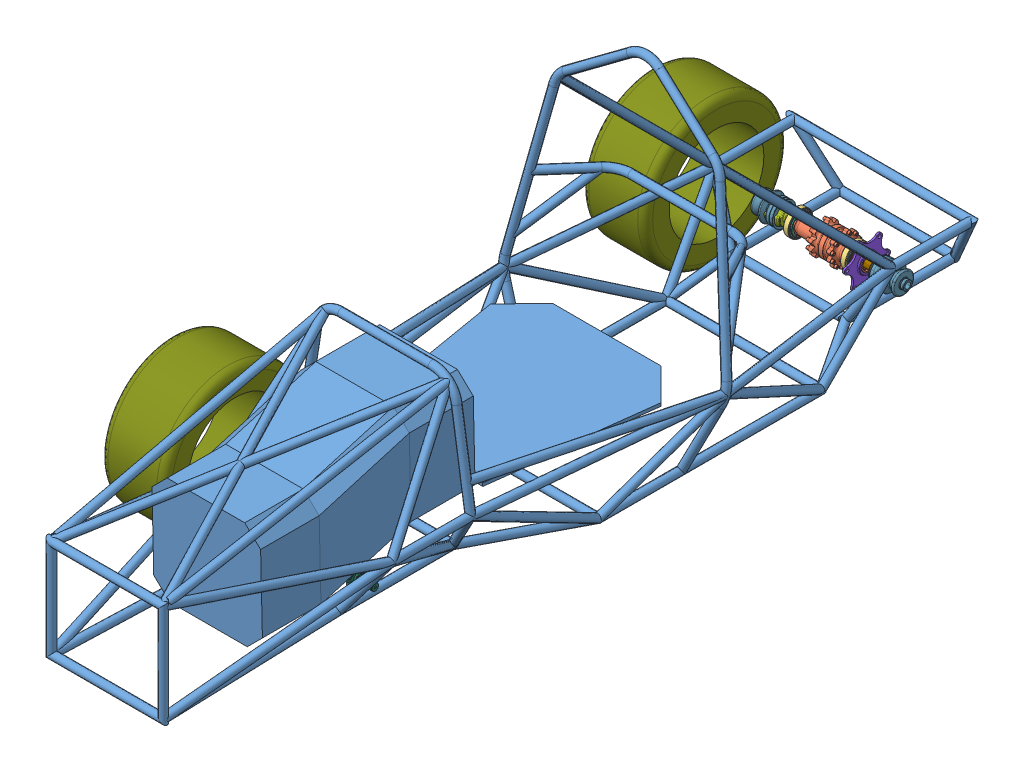
SolidWorks assembly ASSEM_Base_Suspension, configuration Default. Lengths in mm.
Overall size (982.83 1092.76 2583.29).
261 component instances, 16 part files, 10 mates.
Components (placement in the parent):
- 2024_Chassis_V1_RevA-1: 2024_Chassis_V1_RevA [Default<As Machined>] at origin size (743.23 992.29 2569.32)
- Differential Assembly-1: Differential Assembly [Default] at (-98.7457 437.9567 -745.2888) x (1 0 0) z (0 -0.960953 -0.276711) size (486.11 199.53 196.01)
  - Drexler Differential-1: Drexler Differential [Default] at (98.7457 177.1174 168.5551) x (0 0.999802 -0.019913) z (0 0.019913 0.999802) size (100 234.25 100)
  - SKF_32010 X-1: SKF_32010 X [Default] at (175.1207 177.1174 168.5551) x (-1 0 0) z (0 -0.454274 -0.890862) size (21.27 80 80)
    - 32010 X_or-1: 32010 X_or [Default] x (1 0 0) z (0 0 -1) size (15.5 80 80)
    - 32010 X_r-1: 32010 X_r [Default] x (1 0 0) z (0 -0.24869 -0.968583) size (15.81 10.45 7.5)
    - 32010 X_r-2: 32010 X_r [Default] x (1 0 0) z (0 -0.481754 -0.876307) size (15.81 10.45 7.5)
    - 32010 X_r-3: 32010 X_r [Default] x (1 0 0) z (0 -0.684547 -0.728969) size (15.81 10.45 7.5)
    - 32010 X_r-4: 32010 X_r [Default] x (1 0 0) z (0 -0.844328 -0.535827) size (15.81 10.45 7.5)
    - 32010 X_r-5: 32010 X_r [Default] x (1 0 0) z (0 -0.951057 -0.309017) size (15.81 10.45 7.5)
    - 32010 X_r-6: 32010 X_r [Default] x (1 0 0) z (0 -0.998027 -0.062791) size (15.81 10.45 7.5)
    - 32010 X_r-7: 32010 X_r [Default] x (1 0 0) z (0 -0.982287 0.187381) size (15.81 10.45 7.5)
    - 32010 X_r-8: 32010 X_r [Default] x (1 0 0) z (0 -0.904827 0.425779) size (15.81 10.45 7.5)
    - 32010 X_r-9: 32010 X_r [Default] x (1 0 0) z (0 -0.770513 0.637424) size (15.81 10.45 7.5)
    - 32010 X_r-10: 32010 X_r [Default] x (1 0 0) z (0 -0.587785 0.809017) size (15.81 10.45 7.5)
    - 32010 X_r-11: 32010 X_r [Default] x (1 0 0) z (0 -0.368125 0.929776) size (15.81 10.45 7.5)
    - 32010 X_r-12: 32010 X_r [Default] x (1 0 0) z (0 -0.125333 0.992115) size (15.81 10.45 7.5)
    - 32010 X_r-13: 32010 X_r [Default] x (1 0 0) z (0 0.125333 0.992115) size (15.81 10.45 7.5)
    - 32010 X_r-14: 32010 X_r [Default] x (1 0 0) z (0 0.368125 0.929776) size (15.81 10.45 7.5)
    - 32010 X_r-15: 32010 X_r [Default] x (1 0 0) z (0 0.587785 0.809017) size (15.81 10.45 7.5)
    - 32010 X_r-16: 32010 X_r [Default] x (1 0 0) z (0 0.770513 0.637424) size (15.81 10.45 7.5)
    - 32010 X_r-17: 32010 X_r [Default] x (1 0 0) z (0 0.904827 0.425779) size (15.81 10.45 7.5)
    - 32010 X_r-18: 32010 X_r [Default] x (1 0 0) z (0 0.982287 0.187381) size (15.81 10.45 7.5)
    - 32010 X_r-19: 32010 X_r [Default] x (1 0 0) z (0 0.998027 -0.062791) size (15.81 10.45 7.5)
    - 32010 X_r-20: 32010 X_r [Default] x (1 0 0) z (0 0.951057 -0.309017) size (15.81 10.45 7.5)
    - 32010 X_r-21: 32010 X_r [Default] x (1 0 0) z (0 0.844328 -0.535827) size (15.81 10.45 7.5)
    - 32010 X_r-22: 32010 X_r [Default] x (1 0 0) z (0 0.684547 -0.728969) size (15.81 10.45 7.5)
    - 32010 X_r-23: 32010 X_r [Default] x (1 0 0) z (0 0.481754 -0.876307) size (15.81 10.45 7.5)
    - 32010 X_r-24: 32010 X_r [Default] x (1 0 0) z (0 0.24869 -0.968583) size (15.81 10.45 7.5)
    - 32010 X_r-25: 32010 X_r [Default] x (1 0 0) z (0 0 -1) size (15.81 10.45 7.5)
    - 32010 X_cage-1: 32010 X_cage [Default] x (1 0 0) z (0 0 -1) size (18.02 76.15 76.15)
    - 32010 X_ir-1: 32010 X_ir [Default] x (1 0 0) z (0 0 -1) size (20 65.95 65.95)
  - SKF_32010 X-2: SKF_32010 X [Default] at (-24.8793 177.1174 168.5551) x (1 0 0) z (0 0.890912 0.454177) size (21.27 80 80)
    - 32010 X_or-1: 32010 X_or [Default] x (1 0 0) z (0 0 -1) size (15.5 80 80)
    - 32010 X_r-1: 32010 X_r [Default] x (1 0 0) z (0 -0.24869 -0.968583) size (15.81 10.45 7.5)
    - 32010 X_r-2: 32010 X_r [Default] x (1 0 0) z (0 -0.481754 -0.876307) size (15.81 10.45 7.5)
    - 32010 X_r-3: 32010 X_r [Default] x (1 0 0) z (0 -0.684547 -0.728969) size (15.81 10.45 7.5)
    - 32010 X_r-4: 32010 X_r [Default] x (1 0 0) z (0 -0.844328 -0.535827) size (15.81 10.45 7.5)
    - 32010 X_r-5: 32010 X_r [Default] x (1 0 0) z (0 -0.951057 -0.309017) size (15.81 10.45 7.5)
    - 32010 X_r-6: 32010 X_r [Default] x (1 0 0) z (0 -0.998027 -0.062791) size (15.81 10.45 7.5)
    - 32010 X_r-7: 32010 X_r [Default] x (1 0 0) z (0 -0.982287 0.187381) size (15.81 10.45 7.5)
    - 32010 X_r-8: 32010 X_r [Default] x (1 0 0) z (0 -0.904827 0.425779) size (15.81 10.45 7.5)
    - 32010 X_r-9: 32010 X_r [Default] x (1 0 0) z (0 -0.770513 0.637424) size (15.81 10.45 7.5)
    - 32010 X_r-10: 32010 X_r [Default] x (1 0 0) z (0 -0.587785 0.809017) size (15.81 10.45 7.5)
    - 32010 X_r-11: 32010 X_r [Default] x (1 0 0) z (0 -0.368125 0.929776) size (15.81 10.45 7.5)
    - 32010 X_r-12: 32010 X_r [Default] x (1 0 0) z (0 -0.125333 0.992115) size (15.81 10.45 7.5)
    - 32010 X_r-13: 32010 X_r [Default] x (1 0 0) z (0 0.125333 0.992115) size (15.81 10.45 7.5)
    - 32010 X_r-14: 32010 X_r [Default] x (1 0 0) z (0 0.368125 0.929776) size (15.81 10.45 7.5)
    - 32010 X_r-15: 32010 X_r [Default] x (1 0 0) z (0 0.587785 0.809017) size (15.81 10.45 7.5)
    - 32010 X_r-16: 32010 X_r [Default] x (1 0 0) z (0 0.770513 0.637424) size (15.81 10.45 7.5)
    - 32010 X_r-17: 32010 X_r [Default] x (1 0 0) z (0 0.904827 0.425779) size (15.81 10.45 7.5)
    - 32010 X_r-18: 32010 X_r [Default] x (1 0 0) z (0 0.982287 0.187381) size (15.81 10.45 7.5)
    - 32010 X_r-19: 32010 X_r [Default] x (1 0 0) z (0 0.998027 -0.062791) size (15.81 10.45 7.5)
    - 32010 X_r-20: 32010 X_r [Default] x (1 0 0) z (0 0.951057 -0.309017) size (15.81 10.45 7.5)
    - 32010 X_r-21: 32010 X_r [Default] x (1 0 0) z (0 0.844328 -0.535827) size (15.81 10.45 7.5)
    - 32010 X_r-22: 32010 X_r [Default] x (1 0 0) z (0 0.684547 -0.728969) size (15.81 10.45 7.5)
    - 32010 X_r-23: 32010 X_r [Default] x (1 0 0) z (0 0.481754 -0.876307) size (15.81 10.45 7.5)
    - 32010 X_r-24: 32010 X_r [Default] x (1 0 0) z (0 0.24869 -0.968583) size (15.81 10.45 7.5)
    - 32010 X_r-25: 32010 X_r [Default] x (1 0 0) z (0 0 -1) size (15.81 10.45 7.5)
    - 32010 X_cage-1: 32010 X_cage [Default] x (1 0 0) z (0 0 -1) size (18.02 76.15 76.15)
    - 32010 X_ir-1: 32010 X_ir [Default] x (1 0 0) z (0 0 -1) size (20 65.95 65.95)
  - D4825 (Drexler Long Tripod Housing)-1: D4825 (Drexler Long Tripod Housing) [Default] at (63.1207 177.1174 168.5551) x (0 0.049326 -0.998783) z (-1 0 0) size (65.36 60.36 166.5)
  - SPIDER_DIFFERENTIAL_ADAPTER-1: SPIDER_DIFFERENTIAL_ADAPTER [Default] at (197.8207 177.0374 168.5892) x (0 -0.59882 0.800884) z (-1 0 0) size (132.58 150 27.1)
  - D4824 (Drexler Medium tripod Housing)-1: D4824 (Drexler Medium tripod Housing) [Default] at (134.3707 177.1174 168.5551) x (0 0.677852 0.735198) z (1 0 0) size (65.36 60.36 155.07)
  - D4672-TA (Tripod)-1: D4672-TA (Tripod) [Default] at (321.1307 160.1151 157.3971) x (1 0 0) z (0 0.676209 0.73671) size (25.48 50.64 55.63)
    - D4672-TA.STEP-1: D4672-TA.STEP [Default] at origin size (25.48 50.64 55.63)
      - FSAE Tripod V2.STEP-1: FSAE Tripod V2.STEP [Default] at (-43.6945 4.946 19.6967) size (24.01 46.11 52.87)
      - FSAE roller_2451.STEP-1: FSAE roller_2451.STEP [Default] at (-43.6945 -7.4365 -1.7504) x (0 0.5 0.866025) z (-1 0 0) size (8.74 25.48 25.48)
      - FSAE roller_2451.STEP-2: FSAE roller_2451.STEP [Default] at (-43.6945 -7.4365 41.1438) x (0 0.5 -0.866025) z (1 0 0) size (8.74 25.48 25.48)
      - FSAE roller_2451.STEP-3: FSAE roller_2451.STEP [Default] at (-43.6945 29.711 19.6967) x (0 -1 0) z (-1 0 0) size (8.74 25.48 25.48)
      - needle.STEP-1: needle.STEP [Default] at (-42.3538 -7.5483 -1.6859) x (1 0 0) z (0 0.5 0.866025) size (1.5 1.5 10.16)
      - needle.STEP-2: needle.STEP [Default] at (-42.3574 -7.2961 -1.8314) x (0.976635 0.186114 -0.107453) z (0 0.5 0.866025) size (1.5 1.5 10.16)
      - needle.STEP-3: needle.STEP [Default] at (-42.4235 -7.0506 -1.9732) x (0.907631 0.363531 -0.209884) z (0 0.5 0.866025) size (1.5 1.5 10.16)
      - needle.STEP-4: needle.STEP [Default] at (-42.5489 -6.823 -2.1046) x (0.796213 0.523959 -0.302508) z (0 0.5 0.866025) size (1.5 1.5 10.16)
      - needle.STEP-5: needle.STEP [Default] at (-42.7279 -6.6242 -2.2194) x (0.647588 0.659903 -0.380995) z (0 0.5 0.866025) size (1.5 1.5 10.16)
      - needle.STEP-6: needle.STEP [Default] at (-42.9521 -6.4632 -2.3123) x (0.468701 0.76501 -0.441678) z (0 0.5 0.866025) size (1.5 1.5 10.16)
      - needle.STEP-7: needle.STEP [Default] at (-43.2109 -6.3478 -2.3789) x (0.267911 0.834367 -0.481722) z (0 0.5 0.866025) size (1.5 1.5 10.16)
      - needle.STEP-8: needle.STEP [Default] at (-43.4924 -6.2833 -2.4162) x (0.054602 0.864733 -0.499254) z (0 0.5 0.866025) size (1.5 1.5 10.16)
      - needle.STEP-9: needle.STEP [Default] at (-43.7833 -6.2726 -2.4224) x (-0.161259 0.854691 -0.493456) z (0 0.5 0.866025) size (1.5 1.5 10.16)
      - needle.STEP-10: needle.STEP [Default] at (-44.07 -6.3163 -2.3971) x (-0.369585 0.804708 -0.464599) z (0 0.5 0.866025) size (1.5 1.5 10.16)
      - needle.STEP-11: needle.STEP [Default] at (-44.3392 -6.4124 -2.3417) x (-0.560639 0.717121 -0.41403) z (0 0.5 0.866025) size (1.5 1.5 10.16)
      - needle.STEP-12: needle.STEP [Default] at (-44.5783 -6.5563 -2.2586) x (-0.725495 0.596023 -0.344114) z (0 0.5 0.866025) size (1.5 1.5 10.16)
      - needle.STEP-13: needle.STEP [Default] at (-44.7761 -6.7413 -2.1517) x (-0.856447 0.447072 -0.258117) z (0 0.5 0.866025) size (1.5 1.5 10.16)
      - needle.STEP-14: needle.STEP [Default] at (-44.9233 -6.9589 -2.0261) x (-0.947378 0.277229 -0.160058) z (0 0.5 0.866025) size (1.5 1.5 10.16)
      - needle.STEP-15: needle.STEP [Default] at (-45.0131 -7.1987 -1.8877) x (-0.994037 0.094432 -0.05452) z (0 0.5 0.866025) size (1.5 1.5 10.16)
      - needle.STEP-16: needle.STEP [Default] at (-45.0413 -7.4497 -1.7428) x (-0.994245 -0.092779 0.053566) z (0 0.5 0.866025) size (1.5 1.5 10.16)
      - needle.STEP-17: needle.STEP [Default] at (-45.0065 -7.7 -1.5982) x (-0.947991 -0.275654 0.159149) z (0 0.5 0.866025) size (1.5 1.5 10.16)
      - needle.STEP-18: needle.STEP [Default] at (-44.9105 -7.9381 -1.4608) x (-0.857437 -0.445647 0.257295) z (0 0.5 0.866025) size (1.5 1.5 10.16)
      - needle.STEP-19: needle.STEP [Default] at (-44.7576 -8.1527 -1.3369) x (-0.726814 -0.594816 0.343417) z (0 0.5 0.866025) size (1.5 1.5 10.16)
      - needle.STEP-20: needle.STEP [Default] at (-44.555 -8.3338 -1.2323) x (-0.562228 -0.716188 0.413491) z (0 0.5 0.866025) size (1.5 1.5 10.16)
      - needle.STEP-21: needle.STEP [Default] at (-44.3122 -8.473 -1.152) x (-0.371368 -0.804092 0.464243) z (0 0.5 0.866025) size (1.5 1.5 10.16)
      - needle.STEP-22: needle.STEP [Default] at (-44.0406 -8.5637 -1.0996) x (-0.163154 -0.854421 0.4933) z (0 0.5 0.866025) size (1.5 1.5 10.16)
      - needle.STEP-23: needle.STEP [Default] at (-43.7528 -8.6018 -1.0776) x (0.052685 -0.864823 0.499306) z (0 0.5 0.866025) size (1.5 1.5 10.16)
      - needle.STEP-24: needle.STEP [Default] at (-43.4622 -8.5854 -1.0871) x (0.266061 -0.834811 0.481978) z (0 0.5 0.866025) size (1.5 1.5 10.16)
      - needle.STEP-25: needle.STEP [Default] at (-43.1825 -8.5153 -1.1275) x (0.467004 -0.765787 0.442128) z (0 0.5 0.866025) size (1.5 1.5 10.16)
      - needle.STEP-26: needle.STEP [Default] at (-42.9268 -8.3949 -1.1971) x (0.646124 -0.660979 0.381616) z (0 0.5 0.866025) size (1.5 1.5 10.16)
      - needle.STEP-27: needle.STEP [Default] at (-42.7069 -8.2296 -1.2925) x (0.79505 -0.525282 0.303272) z (0 0.5 0.866025) size (1.5 1.5 10.16)
      - needle.STEP-28: needle.STEP [Default] at (-42.5332 -8.0272 -1.4093) x (0.906823 -0.365039 0.210755) z (0 0.5 0.866025) size (1.5 1.5 10.16)
      - needle.STEP-29: needle.STEP [Default] at (-42.4137 -7.7973 -1.5421) x (0.97622 -0.187737 0.10839) z (0 0.5 0.866025) size (1.5 1.5 10.16)
      - needle.STEP-30: needle.STEP [Default] at (-42.3538 29.711 19.5676) x (1 0 0) z (0 -1 0) size (1.5 1.5 10.16)
      - needle.STEP-31: needle.STEP [Default] at (-42.3538 -7.3247 41.2084) x (1 0 0) z (0 0.5 -0.866025) size (1.5 1.5 10.16)
      - needle.STEP-32: needle.STEP [Default] at (-42.4137 29.711 19.2801) x (0.97622 0 -0.21678) z (0 -1 0) size (1.5 1.5 10.16)
      - needle.STEP-33: needle.STEP [Default] at (-42.4137 -7.0756 41.3522) x (0.97622 0.187737 0.10839) z (0 0.5 -0.866025) size (1.5 1.5 10.16)
      - needle.STEP-34: needle.STEP [Default] at (-42.5332 29.711 19.0146) x (0.906823 0 -0.421511) z (0 -1 0) size (1.5 1.5 10.16)
      - needle.STEP-35: needle.STEP [Default] at (-42.5332 -6.8457 41.4849) x (0.906823 0.365039 0.210755) z (0 0.5 -0.866025) size (1.5 1.5 10.16)
      - needle.STEP-36: needle.STEP [Default] at (-42.7069 29.711 18.7809) x (0.79505 0 -0.606544) z (0 -1 0) size (1.5 1.5 10.16)
      - needle.STEP-37: needle.STEP [Default] at (-42.7069 -6.6434 41.6017) x (0.79505 0.525282 0.303272) z (0 0.5 -0.866025) size (1.5 1.5 10.16)
      - needle.STEP-38: needle.STEP [Default] at (-42.9268 29.711 18.5901) x (0.646124 0 -0.763232) z (0 -1 0) size (1.5 1.5 10.16)
      - needle.STEP-39: needle.STEP [Default] at (-42.9268 -6.4781 41.6972) x (0.646124 0.660979 0.381616) z (0 0.5 -0.866025) size (1.5 1.5 10.16)
      - needle.STEP-40: needle.STEP [Default] at (-43.1825 29.711 18.4509) x (0.467004 0 -0.884255) z (0 -1 0) size (1.5 1.5 10.16)
      - needle.STEP-41: needle.STEP [Default] at (-43.1825 -6.3576 41.7667) x (0.467004 0.765787 0.442128) z (0 0.5 -0.866025) size (1.5 1.5 10.16)
      - needle.STEP-42: needle.STEP [Default] at (-43.4622 29.711 18.37) x (0.266061 0 -0.963956) z (0 -1 0) size (1.5 1.5 10.16)
      - needle.STEP-43: needle.STEP [Default] at (-43.4622 -6.2875 41.8072) x (0.266061 0.834811 0.481978) z (0 0.5 -0.866025) size (1.5 1.5 10.16)
      - needle.STEP-44: needle.STEP [Default] at (-43.7528 29.711 18.3511) x (0.052685 0 -0.998611) z (0 -1 0) size (1.5 1.5 10.16)
      - needle.STEP-45: needle.STEP [Default] at (-43.7528 -6.2711 41.8166) x (0.052685 0.864823 0.499306) z (0 0.5 -0.866025) size (1.5 1.5 10.16)
      - needle.STEP-46: needle.STEP [Default] at (-44.0406 29.711 18.3951) x (-0.163154 0 -0.986601) z (0 -1 0) size (1.5 1.5 10.16)
      - needle.STEP-47: needle.STEP [Default] at (-44.0406 -6.3092 41.7947) x (-0.163154 0.854421 0.4933) z (0 0.5 -0.866025) size (1.5 1.5 10.16)
      - needle.STEP-48: needle.STEP [Default] at (-44.3122 29.711 18.4999) x (-0.371368 0 -0.928486) z (0 -1 0) size (1.5 1.5 10.16)
      - needle.STEP-49: needle.STEP [Default] at (-44.3122 -6.4 41.7423) x (-0.371368 0.804092 0.464243) z (0 0.5 -0.866025) size (1.5 1.5 10.16)
      - needle.STEP-50: needle.STEP [Default] at (-44.555 29.711 18.6606) x (-0.562228 0 -0.826982) z (0 -1 0) size (1.5 1.5 10.16)
      - needle.STEP-51: needle.STEP [Default] at (-44.555 -6.5392 41.6619) x (-0.562228 0.716188 0.413491) z (0 0.5 -0.866025) size (1.5 1.5 10.16)
      - needle.STEP-52: needle.STEP [Default] at (-44.7576 29.711 18.8697) x (-0.726814 0 -0.686834) z (0 -1 0) size (1.5 1.5 10.16)
      - needle.STEP-53: needle.STEP [Default] at (-44.7576 -6.7203 41.5573) x (-0.726814 0.594816 0.343417) z (0 0.5 -0.866025) size (1.5 1.5 10.16)
      - needle.STEP-54: needle.STEP [Default] at (-44.9105 29.711 19.1175) x (-0.857437 0 -0.514589) z (0 -1 0) size (1.5 1.5 10.16)
      - needle.STEP-55: needle.STEP [Default] at (-44.9105 -6.9349 41.4334) x (-0.857437 0.445647 0.257295) z (0 0.5 -0.866025) size (1.5 1.5 10.16)
      - needle.STEP-56: needle.STEP [Default] at (-45.0065 29.711 19.3924) x (-0.947991 0 -0.318298) z (0 -1 0) size (1.5 1.5 10.16)
      - needle.STEP-57: needle.STEP [Default] at (-45.0065 -7.1729 41.296) x (-0.947991 0.275654 0.159149) z (0 0.5 -0.866025) size (1.5 1.5 10.16)
      - needle.STEP-58: needle.STEP [Default] at (-45.0413 29.711 19.6814) x (-0.994245 0 -0.107132) z (0 -1 0) size (1.5 1.5 10.16)
      - needle.STEP-59: needle.STEP [Default] at (-45.0413 -7.4232 41.1515) x (-0.994245 0.092779 0.053566) z (0 0.5 -0.866025) size (1.5 1.5 10.16)
      - needle.STEP-60: needle.STEP [Default] at (-45.0131 29.711 19.9712) x (-0.994037 0 0.10904) z (0 -1 0) size (1.5 1.5 10.16)
      - needle.STEP-61: needle.STEP [Default] at (-45.0131 -7.6742 41.0066) x (-0.994037 -0.094432 -0.05452) z (0 0.5 -0.866025) size (1.5 1.5 10.16)
      - needle.STEP-62: needle.STEP [Default] at (-44.9233 29.711 20.2482) x (-0.947378 0 0.320117) z (0 -1 0) size (1.5 1.5 10.16)
      - needle.STEP-63: needle.STEP [Default] at (-44.9233 -7.914 40.8681) x (-0.947378 -0.277229 -0.160058) z (0 0.5 -0.866025) size (1.5 1.5 10.16)
      - needle.STEP-64: needle.STEP [Default] at (-44.7761 29.711 20.4994) x (-0.856447 0 0.516234) z (0 -1 0) size (1.5 1.5 10.16)
      - needle.STEP-65: needle.STEP [Default] at (-44.7761 -8.1316 40.7425) x (-0.856447 -0.447072 -0.258117) z (0 0.5 -0.866025) size (1.5 1.5 10.16)
      - needle.STEP-66: needle.STEP [Default] at (-44.5783 29.711 20.7131) x (-0.725495 0 0.688228) z (0 -1 0) size (1.5 1.5 10.16)
      - needle.STEP-67: needle.STEP [Default] at (-44.5783 -8.3166 40.6357) x (-0.725495 -0.596023 -0.344114) z (0 0.5 -0.866025) size (1.5 1.5 10.16)
      - needle.STEP-68: needle.STEP [Default] at (-44.3392 29.711 20.8792) x (-0.560639 0 0.82806) z (0 -1 0) size (1.5 1.5 10.16)
      - needle.STEP-69: needle.STEP [Default] at (-44.3392 -8.4606 40.5526) x (-0.560639 -0.717121 -0.41403) z (0 0.5 -0.866025) size (1.5 1.5 10.16)
      - needle.STEP-70: needle.STEP [Default] at (-44.07 29.711 20.9902) x (-0.369585 0 0.929197) z (0 -1 0) size (1.5 1.5 10.16)
      - needle.STEP-71: needle.STEP [Default] at (-44.07 -8.5566 40.4971) x (-0.369585 -0.804708 -0.464599) z (0 0.5 -0.866025) size (1.5 1.5 10.16)
      - needle.STEP-72: needle.STEP [Default] at (-43.7833 29.711 21.0407) x (-0.161259 0 0.986912) z (0 -1 0) size (1.5 1.5 10.16)
      - needle.STEP-73: needle.STEP [Default] at (-43.7833 -8.6003 40.4719) x (-0.161259 -0.854691 -0.493456) z (0 0.5 -0.866025) size (1.5 1.5 10.16)
      - needle.STEP-74: needle.STEP [Default] at (-43.4924 29.711 21.0283) x (0.054602 0 0.998508) z (0 -1 0) size (1.5 1.5 10.16)
      - needle.STEP-75: needle.STEP [Default] at (-43.4924 -8.5897 40.478) x (0.054602 -0.864733 -0.499254) z (0 0.5 -0.866025) size (1.5 1.5 10.16)
      - needle.STEP-76: needle.STEP [Default] at (-43.2109 29.711 20.9538) x (0.267911 0 0.963444) z (0 -1 0) size (1.5 1.5 10.16)
      - needle.STEP-77: needle.STEP [Default] at (-43.2109 -8.5251 40.5153) x (0.267911 -0.834367 -0.481722) z (0 0.5 -0.866025) size (1.5 1.5 10.16)
      - needle.STEP-78: needle.STEP [Default] at (-42.9521 29.711 20.8205) x (0.468701 0 0.883357) z (0 -1 0) size (1.5 1.5 10.16)
      - needle.STEP-79: needle.STEP [Default] at (-42.9521 -8.4097 40.582) x (0.468701 -0.76501 -0.441678) z (0 0.5 -0.866025) size (1.5 1.5 10.16)
      - needle.STEP-80: needle.STEP [Default] at (-42.7279 29.711 20.6347) x (0.647588 0 0.761991) z (0 -1 0) size (1.5 1.5 10.16)
      - needle.STEP-81: needle.STEP [Default] at (-42.7279 -8.2488 40.6749) x (0.647588 -0.659903 -0.380995) z (0 0.5 -0.866025) size (1.5 1.5 10.16)
      - needle.STEP-82: needle.STEP [Default] at (-42.5489 29.711 20.4051) x (0.796213 0 0.605016) z (0 -1 0) size (1.5 1.5 10.16)
      - needle.STEP-83: needle.STEP [Default] at (-42.5489 -8.0499 40.7897) x (0.796213 -0.523959 -0.302508) z (0 0.5 -0.866025) size (1.5 1.5 10.16)
      - needle.STEP-84: needle.STEP [Default] at (-42.4235 29.711 20.1423) x (0.907631 0 0.419769) z (0 -1 0) size (1.5 1.5 10.16)
      - needle.STEP-85: needle.STEP [Default] at (-42.4235 -7.8224 40.921) x (0.907631 -0.363531 -0.209884) z (0 0.5 -0.866025) size (1.5 1.5 10.16)
      - needle.STEP-86: needle.STEP [Default] at (-42.3574 29.711 19.8588) x (0.976635 0 0.214906) z (0 -1 0) size (1.5 1.5 10.16)
      - needle.STEP-87: needle.STEP [Default] at (-42.3574 -7.5768 41.0628) x (0.976635 -0.186114 -0.107453) z (0 0.5 -0.866025) size (1.5 1.5 10.16)
      - Tripod Retainer.STEP-1: Tripod Retainer.STEP [Default] at (-43.6945 -8.0715 -2.8502) x (0.973299 0.198788 -0.11477) z (0 0.5 0.866025) size (15.88 15.88 1.27)
      - Tripod Retainer.STEP-2: Tripod Retainer.STEP [Default] at (-43.6945 -8.0715 42.2437) x (0.973299 -0.198788 -0.11477) z (0 0.5 -0.866025) size (15.88 15.88 1.27)
      - Tripod Retainer.STEP-3: Tripod Retainer.STEP [Default] at (-43.6945 30.981 19.6967) x (0.973299 0 0.229541) z (0 -1 0) size (15.88 15.88 1.27)
  - D4672-TA (Tripod)-2: D4672-TA (Tripod) [Default] at (-47.6803 161.7899 181.8937) x (1 0 0) z (0 0.890652 -0.454686) size (25.48 50.64 55.63)
    - D4672-TA.STEP-1: D4672-TA.STEP [Default] at origin size (25.48 50.64 55.63)
      - FSAE Tripod V2.STEP-1: FSAE Tripod V2.STEP [Default] at (-43.6945 4.946 19.6967) size (24.01 46.11 52.87)
      - FSAE roller_2451.STEP-1: FSAE roller_2451.STEP [Default] at (-43.6945 -7.4365 -1.7504) x (0 0.5 0.866025) z (-1 0 0) size (8.74 25.48 25.48)
      - FSAE roller_2451.STEP-2: FSAE roller_2451.STEP [Default] at (-43.6945 -7.4365 41.1438) x (0 0.5 -0.866025) z (1 0 0) size (8.74 25.48 25.48)
      - FSAE roller_2451.STEP-3: FSAE roller_2451.STEP [Default] at (-43.6945 29.711 19.6967) x (0 -1 0) z (-1 0 0) size (8.74 25.48 25.48)
      - needle.STEP-1: needle.STEP [Default] at (-42.3538 -7.5483 -1.6859) x (1 0 0) z (0 0.5 0.866025) size (1.5 1.5 10.16)
      - needle.STEP-2: needle.STEP [Default] at (-42.3574 -7.2961 -1.8314) x (0.976635 0.186114 -0.107453) z (0 0.5 0.866025) size (1.5 1.5 10.16)
      - needle.STEP-3: needle.STEP [Default] at (-42.4235 -7.0506 -1.9732) x (0.907631 0.363531 -0.209884) z (0 0.5 0.866025) size (1.5 1.5 10.16)
      - needle.STEP-4: needle.STEP [Default] at (-42.5489 -6.823 -2.1046) x (0.796213 0.523959 -0.302508) z (0 0.5 0.866025) size (1.5 1.5 10.16)
      - needle.STEP-5: needle.STEP [Default] at (-42.7279 -6.6242 -2.2194) x (0.647588 0.659903 -0.380995) z (0 0.5 0.866025) size (1.5 1.5 10.16)
      - needle.STEP-6: needle.STEP [Default] at (-42.9521 -6.4632 -2.3123) x (0.468701 0.76501 -0.441678) z (0 0.5 0.866025) size (1.5 1.5 10.16)
      - needle.STEP-7: needle.STEP [Default] at (-43.2109 -6.3478 -2.3789) x (0.267911 0.834367 -0.481722) z (0 0.5 0.866025) size (1.5 1.5 10.16)
      - needle.STEP-8: needle.STEP [Default] at (-43.4924 -6.2833 -2.4162) x (0.054602 0.864733 -0.499254) z (0 0.5 0.866025) size (1.5 1.5 10.16)
      - needle.STEP-9: needle.STEP [Default] at (-43.7833 -6.2726 -2.4224) x (-0.161259 0.854691 -0.493456) z (0 0.5 0.866025) size (1.5 1.5 10.16)
      - needle.STEP-10: needle.STEP [Default] at (-44.07 -6.3163 -2.3971) x (-0.369585 0.804708 -0.464599) z (0 0.5 0.866025) size (1.5 1.5 10.16)
      - needle.STEP-11: needle.STEP [Default] at (-44.3392 -6.4124 -2.3417) x (-0.560639 0.717121 -0.41403) z (0 0.5 0.866025) size (1.5 1.5 10.16)
      - needle.STEP-12: needle.STEP [Default] at (-44.5783 -6.5563 -2.2586) x (-0.725495 0.596023 -0.344114) z (0 0.5 0.866025) size (1.5 1.5 10.16)
      - needle.STEP-13: needle.STEP [Default] at (-44.7761 -6.7413 -2.1517) x (-0.856447 0.447072 -0.258117) z (0 0.5 0.866025) size (1.5 1.5 10.16)
      - needle.STEP-14: needle.STEP [Default] at (-44.9233 -6.9589 -2.0261) x (-0.947378 0.277229 -0.160058) z (0 0.5 0.866025) size (1.5 1.5 10.16)
      - needle.STEP-15: needle.STEP [Default] at (-45.0131 -7.1987 -1.8877) x (-0.994037 0.094432 -0.05452) z (0 0.5 0.866025) size (1.5 1.5 10.16)
      - needle.STEP-16: needle.STEP [Default] at (-45.0413 -7.4497 -1.7428) x (-0.994245 -0.092779 0.053566) z (0 0.5 0.866025) size (1.5 1.5 10.16)
      - needle.STEP-17: needle.STEP [Default] at (-45.0065 -7.7 -1.5982) x (-0.947991 -0.275654 0.159149) z (0 0.5 0.866025) size (1.5 1.5 10.16)
      - needle.STEP-18: needle.STEP [Default] at (-44.9105 -7.9381 -1.4608) x (-0.857437 -0.445647 0.257295) z (0 0.5 0.866025) size (1.5 1.5 10.16)
      - needle.STEP-19: needle.STEP [Default] at (-44.7576 -8.1527 -1.3369) x (-0.726814 -0.594816 0.343417) z (0 0.5 0.866025) size (1.5 1.5 10.16)
      - needle.STEP-20: needle.STEP [Default] at (-44.555 -8.3338 -1.2323) x (-0.562228 -0.716188 0.413491) z (0 0.5 0.866025) size (1.5 1.5 10.16)
      - needle.STEP-21: needle.STEP [Default] at (-44.3122 -8.473 -1.152) x (-0.371368 -0.804092 0.464243) z (0 0.5 0.866025) size (1.5 1.5 10.16)
      - needle.STEP-22: needle.STEP [Default] at (-44.0406 -8.5637 -1.0996) x (-0.163154 -0.854421 0.4933) z (0 0.5 0.866025) size (1.5 1.5 10.16)
      - needle.STEP-23: needle.STEP [Default] at (-43.7528 -8.6018 -1.0776) x (0.052685 -0.864823 0.499306) z (0 0.5 0.866025) size (1.5 1.5 10.16)
      - needle.STEP-24: needle.STEP [Default] at (-43.4622 -8.5854 -1.0871) x (0.266061 -0.834811 0.481978) z (0 0.5 0.866025) size (1.5 1.5 10.16)
      - needle.STEP-25: needle.STEP [Default] at (-43.1825 -8.5153 -1.1275) x (0.467004 -0.765787 0.442128) z (0 0.5 0.866025) size (1.5 1.5 10.16)
      - needle.STEP-26: needle.STEP [Default] at (-42.9268 -8.3949 -1.1971) x (0.646124 -0.660979 0.381616) z (0 0.5 0.866025) size (1.5 1.5 10.16)
      - needle.STEP-27: needle.STEP [Default] at (-42.7069 -8.2296 -1.2925) x (0.79505 -0.525282 0.303272) z (0 0.5 0.866025) size (1.5 1.5 10.16)
      - needle.STEP-28: needle.STEP [Default] at (-42.5332 -8.0272 -1.4093) x (0.906823 -0.365039 0.210755) z (0 0.5 0.866025) size (1.5 1.5 10.16)
      - needle.STEP-29: needle.STEP [Default] at (-42.4137 -7.7973 -1.5421) x (0.97622 -0.187737 0.10839) z (0 0.5 0.866025) size (1.5 1.5 10.16)
      - needle.STEP-30: needle.STEP [Default] at (-42.3538 29.711 19.5676) x (1 0 0) z (0 -1 0) size (1.5 1.5 10.16)
      - needle.STEP-31: needle.STEP [Default] at (-42.3538 -7.3247 41.2084) x (1 0 0) z (0 0.5 -0.866025) size (1.5 1.5 10.16)
      - needle.STEP-32: needle.STEP [Default] at (-42.4137 29.711 19.2801) x (0.97622 0 -0.21678) z (0 -1 0) size (1.5 1.5 10.16)
      - needle.STEP-33: needle.STEP [Default] at (-42.4137 -7.0756 41.3522) x (0.97622 0.187737 0.10839) z (0 0.5 -0.866025) size (1.5 1.5 10.16)
      - needle.STEP-34: needle.STEP [Default] at (-42.5332 29.711 19.0146) x (0.906823 0 -0.421511) z (0 -1 0) size (1.5 1.5 10.16)
      - needle.STEP-35: needle.STEP [Default] at (-42.5332 -6.8457 41.4849) x (0.906823 0.365039 0.210755) z (0 0.5 -0.866025) size (1.5 1.5 10.16)
      - needle.STEP-36: needle.STEP [Default] at (-42.7069 29.711 18.7809) x (0.79505 0 -0.606544) z (0 -1 0) size (1.5 1.5 10.16)
      - needle.STEP-37: needle.STEP [Default] at (-42.7069 -6.6434 41.6017) x (0.79505 0.525282 0.303272) z (0 0.5 -0.866025) size (1.5 1.5 10.16)
      - needle.STEP-38: needle.STEP [Default] at (-42.9268 29.711 18.5901) x (0.646124 0 -0.763232) z (0 -1 0) size (1.5 1.5 10.16)
      - needle.STEP-39: needle.STEP [Default] at (-42.9268 -6.4781 41.6972) x (0.646124 0.660979 0.381616) z (0 0.5 -0.866025) size (1.5 1.5 10.16)
      - needle.STEP-40: needle.STEP [Default] at (-43.1825 29.711 18.4509) x (0.467004 0 -0.884255) z (0 -1 0) size (1.5 1.5 10.16)
      - needle.STEP-41: needle.STEP [Default] at (-43.1825 -6.3576 41.7667) x (0.467004 0.765787 0.442128) z (0 0.5 -0.866025) size (1.5 1.5 10.16)
      - needle.STEP-42: needle.STEP [Default] at (-43.4622 29.711 18.37) x (0.266061 0 -0.963956) z (0 -1 0) size (1.5 1.5 10.16)
      - needle.STEP-43: needle.STEP [Default] at (-43.4622 -6.2875 41.8072) x (0.266061 0.834811 0.481978) z (0 0.5 -0.866025) size (1.5 1.5 10.16)
      - needle.STEP-44: needle.STEP [Default] at (-43.7528 29.711 18.3511) x (0.052685 0 -0.998611) z (0 -1 0) size (1.5 1.5 10.16)
      - needle.STEP-45: needle.STEP [Default] at (-43.7528 -6.2711 41.8166) x (0.052685 0.864823 0.499306) z (0 0.5 -0.866025) size (1.5 1.5 10.16)
      - needle.STEP-46: needle.STEP [Default] at (-44.0406 29.711 18.3951) x (-0.163154 0 -0.986601) z (0 -1 0) size (1.5 1.5 10.16)
      - needle.STEP-47: needle.STEP [Default] at (-44.0406 -6.3092 41.7947) x (-0.163154 0.854421 0.4933) z (0 0.5 -0.866025) size (1.5 1.5 10.16)
      - needle.STEP-48: needle.STEP [Default] at (-44.3122 29.711 18.4999) x (-0.371368 0 -0.928486) z (0 -1 0) size (1.5 1.5 10.16)
      - needle.STEP-49: needle.STEP [Default] at (-44.3122 -6.4 41.7423) x (-0.371368 0.804092 0.464243) z (0 0.5 -0.866025) size (1.5 1.5 10.16)
      - needle.STEP-50: needle.STEP [Default] at (-44.555 29.711 18.6606) x (-0.562228 0 -0.826982) z (0 -1 0) size (1.5 1.5 10.16)
      - needle.STEP-51: needle.STEP [Default] at (-44.555 -6.5392 41.6619) x (-0.562228 0.716188 0.413491) z (0 0.5 -0.866025) size (1.5 1.5 10.16)
      - needle.STEP-52: needle.STEP [Default] at (-44.7576 29.711 18.8697) x (-0.726814 0 -0.686834) z (0 -1 0) size (1.5 1.5 10.16)
      - needle.STEP-53: needle.STEP [Default] at (-44.7576 -6.7203 41.5573) x (-0.726814 0.594816 0.343417) z (0 0.5 -0.866025) size (1.5 1.5 10.16)
      - needle.STEP-54: needle.STEP [Default] at (-44.9105 29.711 19.1175) x (-0.857437 0 -0.514589) z (0 -1 0) size (1.5 1.5 10.16)
      - needle.STEP-55: needle.STEP [Default] at (-44.9105 -6.9349 41.4334) x (-0.857437 0.445647 0.257295) z (0 0.5 -0.866025) size (1.5 1.5 10.16)
      - needle.STEP-56: needle.STEP [Default] at (-45.0065 29.711 19.3924) x (-0.947991 0 -0.318298) z (0 -1 0) size (1.5 1.5 10.16)
      - needle.STEP-57: needle.STEP [Default] at (-45.0065 -7.1729 41.296) x (-0.947991 0.275654 0.159149) z (0 0.5 -0.866025) size (1.5 1.5 10.16)
      - needle.STEP-58: needle.STEP [Default] at (-45.0413 29.711 19.6814) x (-0.994245 0 -0.107132) z (0 -1 0) size (1.5 1.5 10.16)
      - needle.STEP-59: needle.STEP [Default] at (-45.0413 -7.4232 41.1515) x (-0.994245 0.092779 0.053566) z (0 0.5 -0.866025) size (1.5 1.5 10.16)
      - needle.STEP-60: needle.STEP [Default] at (-45.0131 29.711 19.9712) x (-0.994037 0 0.10904) z (0 -1 0) size (1.5 1.5 10.16)
      - needle.STEP-61: needle.STEP [Default] at (-45.0131 -7.6742 41.0066) x (-0.994037 -0.094432 -0.05452) z (0 0.5 -0.866025) size (1.5 1.5 10.16)
      - needle.STEP-62: needle.STEP [Default] at (-44.9233 29.711 20.2482) x (-0.947378 0 0.320117) z (0 -1 0) size (1.5 1.5 10.16)
      - needle.STEP-63: needle.STEP [Default] at (-44.9233 -7.914 40.8681) x (-0.947378 -0.277229 -0.160058) z (0 0.5 -0.866025) size (1.5 1.5 10.16)
      - needle.STEP-64: needle.STEP [Default] at (-44.7761 29.711 20.4994) x (-0.856447 0 0.516234) z (0 -1 0) size (1.5 1.5 10.16)
      - needle.STEP-65: needle.STEP [Default] at (-44.7761 -8.1316 40.7425) x (-0.856447 -0.447072 -0.258117) z (0 0.5 -0.866025) size (1.5 1.5 10.16)
      - needle.STEP-66: needle.STEP [Default] at (-44.5783 29.711 20.7131) x (-0.725495 0 0.688228) z (0 -1 0) size (1.5 1.5 10.16)
      - needle.STEP-67: needle.STEP [Default] at (-44.5783 -8.3166 40.6357) x (-0.725495 -0.596023 -0.344114) z (0 0.5 -0.866025) size (1.5 1.5 10.16)
      - needle.STEP-68: needle.STEP [Default] at (-44.3392 29.711 20.8792) x (-0.560639 0 0.82806) z (0 -1 0) size (1.5 1.5 10.16)
      - needle.STEP-69: needle.STEP [Default] at (-44.3392 -8.4606 40.5526) x (-0.560639 -0.717121 -0.41403) z (0 0.5 -0.866025) size (1.5 1.5 10.16)
      - needle.STEP-70: needle.STEP [Default] at (-44.07 29.711 20.9902) x (-0.369585 0 0.929197) z (0 -1 0) size (1.5 1.5 10.16)
      - needle.STEP-71: needle.STEP [Default] at (-44.07 -8.5566 40.4971) x (-0.369585 -0.804708 -0.464599) z (0 0.5 -0.866025) size (1.5 1.5 10.16)
      - needle.STEP-72: needle.STEP [Default] at (-43.7833 29.711 21.0407) x (-0.161259 0 0.986912) z (0 -1 0) size (1.5 1.5 10.16)
      - needle.STEP-73: needle.STEP [Default] at (-43.7833 -8.6003 40.4719) x (-0.161259 -0.854691 -0.493456) z (0 0.5 -0.866025) size (1.5 1.5 10.16)
      - needle.STEP-74: needle.STEP [Default] at (-43.4924 29.711 21.0283) x (0.054602 0 0.998508) z (0 -1 0) size (1.5 1.5 10.16)
      - needle.STEP-75: needle.STEP [Default] at (-43.4924 -8.5897 40.478) x (0.054602 -0.864733 -0.499254) z (0 0.5 -0.866025) size (1.5 1.5 10.16)
      - needle.STEP-76: needle.STEP [Default] at (-43.2109 29.711 20.9538) x (0.267911 0 0.963444) z (0 -1 0) size (1.5 1.5 10.16)
      - needle.STEP-77: needle.STEP [Default] at (-43.2109 -8.5251 40.5153) x (0.267911 -0.834367 -0.481722) z (0 0.5 -0.866025) size (1.5 1.5 10.16)
      - needle.STEP-78: needle.STEP [Default] at (-42.9521 29.711 20.8205) x (0.468701 0 0.883357) z (0 -1 0) size (1.5 1.5 10.16)
      - needle.STEP-79: needle.STEP [Default] at (-42.9521 -8.4097 40.582) x (0.468701 -0.76501 -0.441678) z (0 0.5 -0.866025) size (1.5 1.5 10.16)
      - needle.STEP-80: needle.STEP [Default] at (-42.7279 29.711 20.6347) x (0.647588 0 0.761991) z (0 -1 0) size (1.5 1.5 10.16)
      - needle.STEP-81: needle.STEP [Default] at (-42.7279 -8.2488 40.6749) x (0.647588 -0.659903 -0.380995) z (0 0.5 -0.866025) size (1.5 1.5 10.16)
      - needle.STEP-82: needle.STEP [Default] at (-42.5489 29.711 20.4051) x (0.796213 0 0.605016) z (0 -1 0) size (1.5 1.5 10.16)
      - needle.STEP-83: needle.STEP [Default] at (-42.5489 -8.0499 40.7897) x (0.796213 -0.523959 -0.302508) z (0 0.5 -0.866025) size (1.5 1.5 10.16)
      - needle.STEP-84: needle.STEP [Default] at (-42.4235 29.711 20.1423) x (0.907631 0 0.419769) z (0 -1 0) size (1.5 1.5 10.16)
      - needle.STEP-85: needle.STEP [Default] at (-42.4235 -7.8224 40.921) x (0.907631 -0.363531 -0.209884) z (0 0.5 -0.866025) size (1.5 1.5 10.16)
      - needle.STEP-86: needle.STEP [Default] at (-42.3574 29.711 19.8588) x (0.976635 0 0.214906) z (0 -1 0) size (1.5 1.5 10.16)
      - needle.STEP-87: needle.STEP [Default] at (-42.3574 -7.5768 41.0628) x (0.976635 -0.186114 -0.107453) z (0 0.5 -0.866025) size (1.5 1.5 10.16)
      - Tripod Retainer.STEP-1: Tripod Retainer.STEP [Default] at (-43.6945 -8.0715 -2.8502) x (0.973299 0.198788 -0.11477) z (0 0.5 0.866025) size (15.88 15.88 1.27)
      - Tripod Retainer.STEP-2: Tripod Retainer.STEP [Default] at (-43.6945 -8.0715 42.2437) x (0.973299 -0.198788 -0.11477) z (0 0.5 -0.866025) size (15.88 15.88 1.27)
      - Tripod Retainer.STEP-3: Tripod Retainer.STEP [Default] at (-43.6945 30.981 19.6967) x (0.973299 0 0.229541) z (0 -1 0) size (15.88 15.88 1.27)
  - 615-3 (Triangular Tripod Housing Boot)-1: 615-3 (Triangular Tripod Housing Boot) [Default] at (336.0855 177.1174 168.5551) x (0 0.694966 -0.719043) z (1 0 0) size (84.51 84.51 88.49)
  - 615-3 (Triangular Tripod Housing Boot)-2: 615-3 (Triangular Tripod Housing Boot) [Default] at (-150.024 177.1174 168.5551) x (0 -0.881387 -0.472395) z (-1 0 0) size (84.51 84.51 88.49)
- KAZ_Steering_Rack_-_Dumb_Solid-1: KAZ_Steering_Rack_-_Dumb_Solid [Default] at (0 198.8947 1049.6828) x (1 0 0) z (0 1 0) size (386.71 91.39 96.37)
- HoosierTyres_43100Slicks-1: HoosierTyres_43100Slicks [Default] at (-403.86 204.47 902.2716) x (0 1 0) z (0 0 1) size (459.74 205.74 459.74)
- HoosierTyres_43100Slicks-2: HoosierTyres_43100Slicks [Default] at (-378.46 204.47 -621.7284) x (0 -1 0) z (0 0 -1) size (459.74 205.74 459.74)
Mates (geometry in assembly coordinates):
- Concentric1: concentric anti-aligned: cylinder of Differential Assembly-1/Drexler Differential-1 through (-121.625 226.9728 -621.7284) axis (1 0 0) radius 25
- Coincident2: coincident: point of Differential Assembly-1/Drexler Differential-1
- Coincident4: coincident anti-aligned: plane of KAZ_Steering_Rack_-_Dumb_Solid-1 through (139.7 173.4947 1079.6167) normal (0 -1 0)
- Coincident5: coincident anti-aligned: plane of KAZ_Steering_Rack_-_Dumb_Solid-1 through (0 198.8947 1049.6828) normal (-1 0 0)
- Tangent1: tangent anti-aligned: cylinder of HoosierTyres_43100Slicks-1 through (-403.86 204.47 902.2716) axis (1 0 0) radius 229.87
- Tangent2: tangent anti-aligned: cylinder of HoosierTyres_43100Slicks-2 through (-378.46 204.47 -621.7284) axis (1 0 0) radius 229.87
- Distance1: distance = 25.4 mm aligned: plane of HoosierTyres_43100Slicks-1 through (-609.6 52.07 902.2716) normal (-1 0 0); plane of HoosierTyres_43100Slicks-2 through (-584.2 356.87 -621.7284) normal (-1 0 0)
- Coincident8: coincident anti-aligned: plane of HoosierTyres_43100Slicks-1 through (-403.86 204.47 902.2716) normal (0 0 1)
- Coincident9: coincident aligned: plane of HoosierTyres_43100Slicks-2 through (-378.46 204.47 -621.7284) normal (0 0 -1)
- Distance3: distance = 609.6 mm anti-aligned: plane of HoosierTyres_43100Slicks-1 through (-609.6 52.07 902.2716) normal (-1 0 0)
